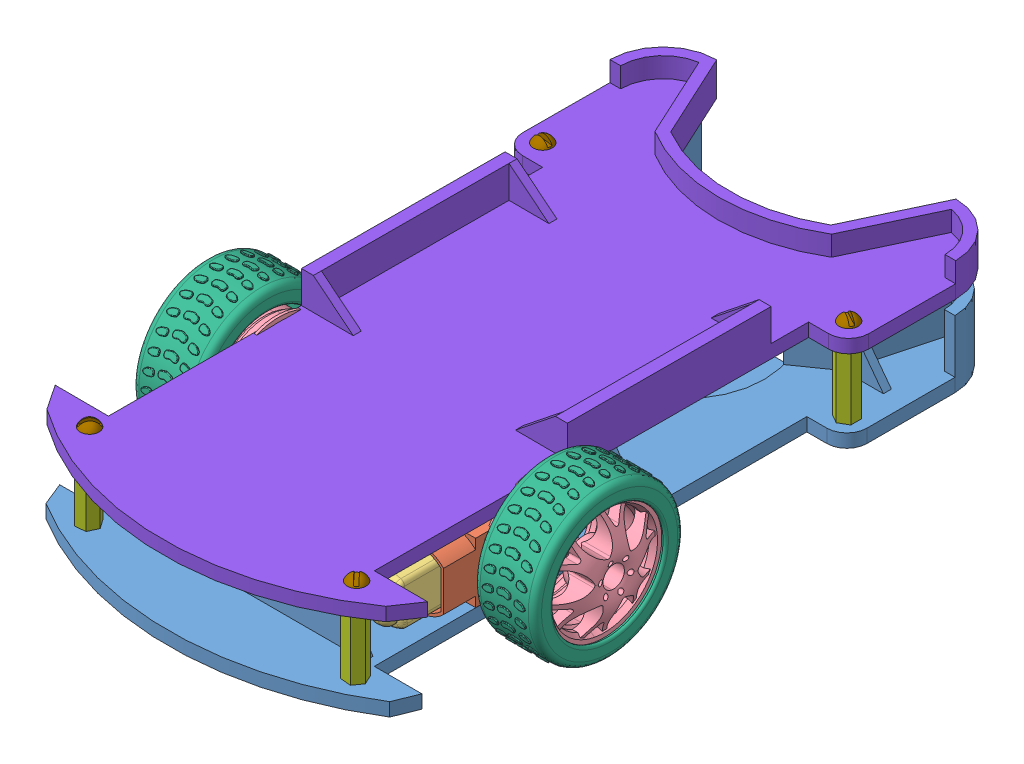
SolidWorks assembly Assembly, configuration Default. Lengths in mm.
Overall size (160.57 74.44 252.19).
20 component instances, 10 part files, 20 mates.
Components (placement in the parent):
- bottom.STEP-3: bottom.STEP [Default] at origin size (135.64 28 246.96)
- motor casing.step-3: motor casing.step [Default] at (-40.72 16.25 24.5) x (0 0 -1) z (1 0 0) size (54 22.64 18.44)
- motor.STEP-1: motor.STEP [Default] at (-42.2141 16.3827 56.5) x (0.996079 -0.088466 0) z (0 0 1) size (11.36 17.01 34.5)
- wheel rim.STEP-1: wheel rim.STEP [Default] at (-60.94 16.2049 18.28) x (1 0 0) z (0 0.982958 -0.183829) size (31.85 43 43)
- shaft.step-1: shaft.step [Default] at (-58.84 16.2049 18.28) x (0 0 -1) z (1 0 0) size (7.2 7.2 18.68)
- new tyre.STEP-1: new tyre.STEP [Default] at (-62.6313 16.2049 18.28) x (1 0 0) z (0 -0.381331 0.924439) size (23 57 57.02)
- new tyre.STEP-2: new tyre.STEP [Default] at (65.2239 16.2049 18.28) x (1 0 0) z (0 -0.381331 0.924439) size (23 57 57.02)
- motor.STEP-2: motor.STEP [Default] at (42.2172 16.383 56.5) x (0.996079 0.088466 0) z (0 0 1) size (11.36 17.01 34.5)
- motor casing.step-4: motor casing.step [Default] at (40.72 16.25 24.5) x (0 0 -1) z (1 0 0) size (54 22.64 18.44)
- wheel rim.STEP-2: wheel rim.STEP [Default] at (60.94 16.2049 18.28) x (-1 0 0) z (0 0.982958 -0.183829) size (31.85 43 43)
- rod.step-1: rod.step [Default] at (-50 5 88) x (0.81659 0 -0.577219) z (0.577219 0 0.81659) size (6.93 26 8)
- rod.step-2: rod.step [Default] at (50 5 88) x (-0.81659 0 -0.577219) z (0.577219 0 -0.81659) size (6.93 26 8)
- rod.step-4: rod.step [Default] at (-57.5 5 -88.5) size (6.93 26 8)
- rod.step-3: rod.step [Default] at (57.5 5 -88.5) x (-1 0 0) z (0 0 -1) size (6.93 26 8)
- top.STEP-1: top.STEP [Default] at (0.3387 31 -0.1916) x (0.999993 0 0.003844) z (-0.003844 0 0.999993) size (140 17 251.65)
- bolt.STEP-1: bolt.STEP [Default] at (-49.9993 30.0324 87.6156) x (-0.738309 0 -0.674462) z (0.674462 0 -0.738309) size (7 14.4 7)
- bolt.STEP-2: bolt.STEP [Default] at (49.9993 30.0324 87.6156) x (0.738309 0 -0.674462) z (0.674462 0 0.738309) size (7 14.4 7)
- bolt.STEP-4: bolt.STEP [Default] at (-56.8207 30.4826 -88.912) x (-0.136983 0 0.990573) z (-0.990573 0 -0.136983) size (7 14.4 7)
- bolt.STEP-3: bolt.STEP [Default] at (58.1785 30.3474 -88.4699) x (-0.47489 0 0.880045) z (-0.880045 0 -0.47489) size (7 14.4 7)
- caster wheel.STEP-2: caster wheel.STEP [Default] at (0 -6.5 -85) x (0.492799 0 0.870143) z (-0.870143 0 0.492799) size (27.5 16.5 27.5)
Mates (geometry in assembly coordinates):
- Concentric6: concentric: cylinder of bottom.step-3 through (-67.82 7.5 38) axis (1 0 0) radius 2.5; cylinder of motor casing.step-3 through (-49.94 7.5 38) axis (1 0 0) radius 1.5
- Concentric7: concentric: cylinder of bottom.step-3 through (-67.82 25 38) axis (1 0 0) radius 2.5; cylinder of motor casing.step-3 through (-49.94 25 38) axis (1 0 0) radius 1.5
- Coincident2: coincident: plane of bottom.step-3 through (-31.5 28 81) normal (-1 0 0); plane of motor casing.step-3 through (-31.5 7 8) normal (1 0 0)
- Concentric8: concentric: circle of motor casing.step-3; line of motor.step-1 through (-40.72 16.25 40) axis (0 0 1)
- Coincident3: coincident: plane of motor casing.step-3 through (-40.72 17.97 44) normal (0 0 1); plane of motor.step-1 through (-41.9064 19.8656 44) normal (0 0 -1)
- Concentric10: concentric: cylinder of motor casing.step-3 through (-57.22 16.25 18) axis (1 0 0) radius 2.75; cylinder of shaft.step-1 through (-40.16 16.25 18) axis (-1 0 0) radius 2.7
- Coincident5: coincident: plane of motor casing.step-3 through (-49.94 7 8) normal (-1 0 0); plane of shaft.step-1 through (-49.94 16.25 18) normal (1 0 0)
- Concentric11: concentric: cylinder of wheel rim.STEP-1 through (-50.94 16.2049 18.28) axis (-1 0 0) radius 2.7; cylinder of shaft.step-1 through (-40.16 16.2049 18.28) axis (-1 0 0) radius 2.7
- Coincident7: coincident: plane of wheel rim.STEP-1 through (-50.94 16.2049 18.28) normal (1 0 0); plane of shaft.step-1 through (-50.94 16.2049 18.28) normal (-1 0 0)
- Concentric13: concentric: cylinder of wheel rim.STEP-1 through (-75.8049 16.2049 18.28) axis (-1 0 0) radius 19; cylinder of new tyre.STEP-1 through (-80.0489 16.2049 18.28) axis (-1 0 0) radius 27
- Concentric14: concentric: cylinder of wheel rim.STEP-1 through (-75.8049 16.2049 18.28) axis (-1 0 0) radius 19; cylinder of new tyre.STEP-1 through (-80.0489 16.2049 18.28) axis (-1 0 0) radius 27
- Concentric15: concentric: circle of bottom.STEP-3; circle of rod.step-1
- Coincident9: coincident: circle of bottom.STEP-3; circle of rod.step-1
- Coincident10: coincident: circle of bottom.STEP-3; circle of rod.STEP-3
- Coincident11: coincident: circle of rod.step-2; circle of top.step-1
- Concentric16: concentric: cylinder of top.STEP-1 through (-49.9993 31 87.6156) axis (0 1 0) radius 2.5; cylinder of bolt.step-1 through (-49.9993 40.3285 87.6156) axis (0 1 0) radius 2
- Lock1: lock: unknown of top.STEP-1; unknown of bolt.STEP-4
- Concentric22: concentric: cylinder of top.STEP-1 through (58.1785 31 -88.4699) axis (0 1 0) radius 2.5; cylinder of bolt.step-3 through (58.1785 40.6435 -88.4699) axis (0 1 0) radius 2
- Concentric27: concentric: circle of bottom.STEP-3; circle of caster wheel.step-2
- Coincident22: coincident: plane of bottom.STEP-3 through (0 0 -14.0415) normal (0 -1 0); plane of caster wheel.step-2 through (0 0 -85) normal (0 1 0)
